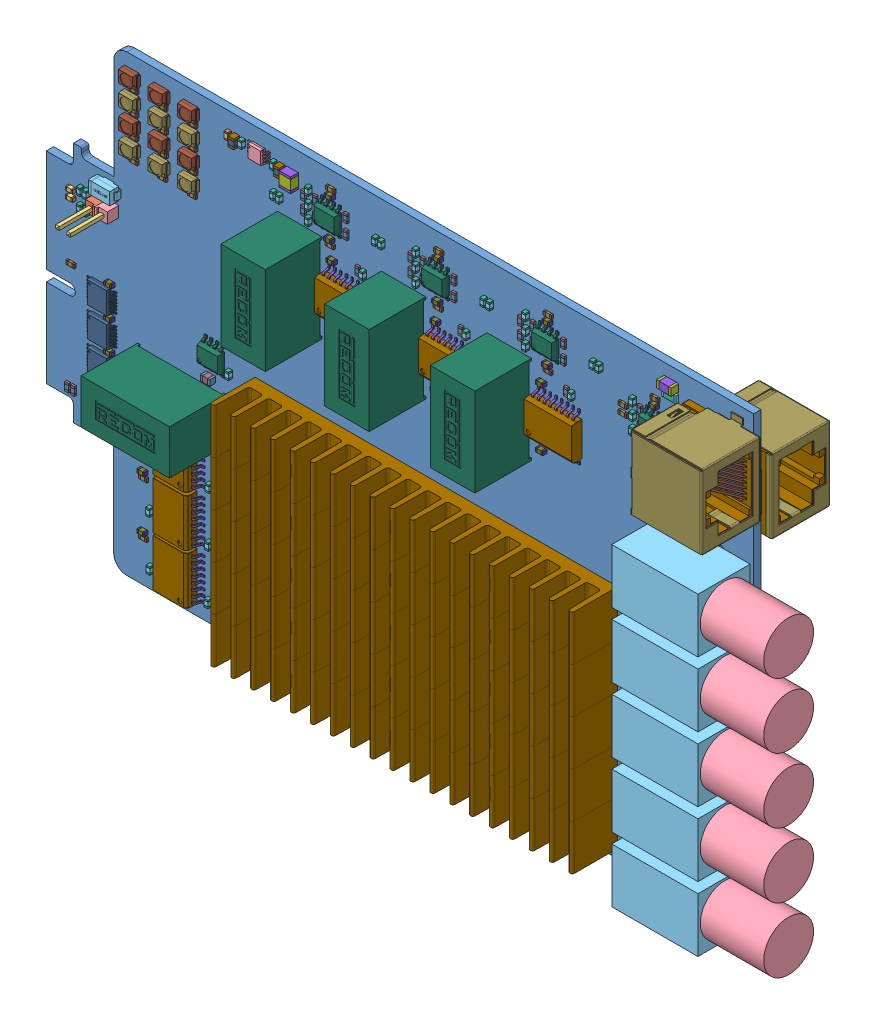
SolidWorks assembly 1166V10, configuration Standard. Lengths in mm.
Overall size (170.01 100 28.53).
2772 component instances, 64 part files, 0 mates.
Components (placement in the parent):
- 1166V10.step-1: 1166V10.step [Standard] at origin size (170.01 100 28.53)
  - Board.step-1: Board.step [Standard] at origin size (155.98 100 1.62)
    - Open CASCADE STEP translator 6.8 1.1.1.step-1: Open CASCADE STEP translator 6.8 1.1.1.step [Standard] at (0 0 -1.622) size (155.98 100 1.62)
  - L103.step-1: L103.step [Standard] at origin size (0.8 1.6 0.8)
    - WE-CBF_0603_CBF.step-1: WE-CBF_0603_CBF.step [Standard] at (40.3999 95.6637 0.4) x (-1 0 0) z (0 0 1) size (0.8 1.6 0.8)
      - L_tende.step-1: L_tende.step [Standard] at (0 -0.5 0) size (0.8 0.3 0.8)
      - L_tende.step-2: L_tende.step [Standard] at (0 0.5 0) x (-1 0 0) z (0 0 1) size (0.8 0.3 0.8)
      - base.step-1: base.step [Standard] at origin size (0.8 1 0.8)
  - IC104.step-1: IC104.step [Standard] at origin size (4.9 3 1.15)
    - MSOP-8.step-1: MSOP-8.step [Standard] at (47.0083 95.5593 0) x (1 0 0) z (0 0 1) size (4.9 3 1.15)
  - CF514.step-1: CF514.step [Standard] at origin size (0.82 1.6 0.9)
    - 6547668352.step-1: 6547668352.step [Standard] at (98.2 92.15 0) size (0.82 0.9 0.9)
      - Extruded.step-1: Extruded.step [Standard] at origin size (0.82 0.9 0.9)
    - 6549602528.step-1: 6549602528.step [Standard] at (98.2 91.525 0) size (0.82 0.35 0.9)
      - Extruded-0.step-1: Extruded-0.step [Standard] at origin size (0.82 0.35 0.9)
    - 6549602528.step-2: 6549602528.step [Standard] at (98.2 92.775 0) size (0.82 0.35 0.9)
      - Extruded-0.step-1: Extruded-0.step [Standard] at origin size (0.82 0.35 0.9)
  - CF513.step-1: CF513.step [Standard] at origin size (0.82 1.6 0.9)
    - 6547668352.step-1: 6547668352.step [Standard] at (96.9 92.15 0) size (0.82 0.9 0.9)
      - Extruded.step-1: Extruded.step [Standard] at origin size (0.82 0.9 0.9)
    - 6549602528.step-1: 6549602528.step [Standard] at (96.9 91.525 0) size (0.82 0.35 0.9)
      - Extruded-0.step-1: Extruded-0.step [Standard] at origin size (0.82 0.35 0.9)
    - 6549602528.step-2: 6549602528.step [Standard] at (96.9 92.775 0) size (0.82 0.35 0.9)
      - Extruded-0.step-1: Extruded-0.step [Standard] at origin size (0.82 0.35 0.9)
  - CF512.step-1: CF512.step [Standard] at origin size (0.82 1.6 0.9)
    - 6547668352.step-1: 6547668352.step [Standard] at (74.3 91.85 0) size (0.82 0.9 0.9)
      - Extruded.step-1: Extruded.step [Standard] at origin size (0.82 0.9 0.9)
    - 6549602528.step-1: 6549602528.step [Standard] at (74.3 91.225 0) size (0.82 0.35 0.9)
      - Extruded-0.step-1: Extruded-0.step [Standard] at origin size (0.82 0.35 0.9)
    - 6549602528.step-2: 6549602528.step [Standard] at (74.3 92.475 0) size (0.82 0.35 0.9)
      - Extruded-0.step-1: Extruded-0.step [Standard] at origin size (0.82 0.35 0.9)
  - CF511.step-1: CF511.step [Standard] at origin size (0.82 1.6 0.9)
    - 6547668352.step-1: 6547668352.step [Standard] at (73 91.85 0) size (0.82 0.9 0.9)
      - Extruded.step-1: Extruded.step [Standard] at origin size (0.82 0.9 0.9)
    - 6549602528.step-1: 6549602528.step [Standard] at (73 91.225 0) size (0.82 0.35 0.9)
      - Extruded-0.step-1: Extruded-0.step [Standard] at origin size (0.82 0.35 0.9)
    - 6549602528.step-2: 6549602528.step [Standard] at (73 92.475 0) size (0.82 0.35 0.9)
      - Extruded-0.step-1: Extruded-0.step [Standard] at origin size (0.82 0.35 0.9)
  - CF510.step-1: CF510.step [Standard] at origin size (0.82 1.6 0.9)
    - 6547668352.step-1: 6547668352.step [Standard] at (122.3 92.25 0) size (0.82 0.9 0.9)
      - Extruded.step-1: Extruded.step [Standard] at origin size (0.82 0.9 0.9)
    - 6549602528.step-1: 6549602528.step [Standard] at (122.3 91.625 0) size (0.82 0.35 0.9)
      - Extruded-0.step-1: Extruded-0.step [Standard] at origin size (0.82 0.35 0.9)
    - 6549602528.step-2: 6549602528.step [Standard] at (122.3 92.875 0) size (0.82 0.35 0.9)
      - Extruded-0.step-1: Extruded-0.step [Standard] at origin size (0.82 0.35 0.9)
  - CF509.step-1: CF509.step [Standard] at origin size (0.82 1.6 0.9)
    - 6547668352.step-1: 6547668352.step [Standard] at (121 92.25 0) size (0.82 0.9 0.9)
      - Extruded.step-1: Extruded.step [Standard] at origin size (0.82 0.9 0.9)
    - 6549602528.step-1: 6549602528.step [Standard] at (121 91.625 0) size (0.82 0.35 0.9)
      - Extruded-0.step-1: Extruded-0.step [Standard] at origin size (0.82 0.35 0.9)
    - 6549602528.step-2: 6549602528.step [Standard] at (121 92.875 0) size (0.82 0.35 0.9)
      - Extruded-0.step-1: Extruded-0.step [Standard] at origin size (0.82 0.35 0.9)
  - CF508.step-1: CF508.step [Standard] at origin size (0.82 1.6 0.9)
    - 6547668352.step-1: 6547668352.step [Standard] at (51.8 89.35 0) size (0.82 0.9 0.9)
      - Extruded.step-1: Extruded.step [Standard] at origin size (0.82 0.9 0.9)
    - 6549602528.step-1: 6549602528.step [Standard] at (51.8 88.725 0) size (0.82 0.35 0.9)
      - Extruded-0.step-1: Extruded-0.step [Standard] at origin size (0.82 0.35 0.9)
    - 6549602528.step-2: 6549602528.step [Standard] at (51.8 89.975 0) size (0.82 0.35 0.9)
      - Extruded-0.step-1: Extruded-0.step [Standard] at origin size (0.82 0.35 0.9)
  - CF507.step-1: CF507.step [Standard] at origin size (0.82 1.6 0.9)
    - 6547668352.step-1: 6547668352.step [Standard] at (50.5 89.35 0) size (0.82 0.9 0.9)
      - Extruded.step-1: Extruded.step [Standard] at origin size (0.82 0.9 0.9)
    - 6549602528.step-1: 6549602528.step [Standard] at (50.5 88.725 0) size (0.82 0.35 0.9)
      - Extruded-0.step-1: Extruded-0.step [Standard] at origin size (0.82 0.35 0.9)
    - 6549602528.step-2: 6549602528.step [Standard] at (50.5 89.975 0) size (0.82 0.35 0.9)
      - Extruded-0.step-1: Extruded-0.step [Standard] at origin size (0.82 0.35 0.9)
  - CF506.step-1: CF506.step [Standard] at origin size (0.82 1.6 0.9)
    - 6549602528.step-1: 6549602528.step [Standard] at (135.1 85.325 -2.522) size (0.82 0.35 0.9)
      - Extruded-0.step-1: Extruded-0.step [Standard] at origin size (0.82 0.35 0.9)
    - 6549602528.step-2: 6549602528.step [Standard] at (135.1 86.575 -2.522) size (0.82 0.35 0.9)
      - Extruded-0.step-1: Extruded-0.step [Standard] at origin size (0.82 0.35 0.9)
    - 6547668352.step-1: 6547668352.step [Standard] at (135.1 85.95 -2.522) size (0.82 0.9 0.9)
      - Extruded.step-1: Extruded.step [Standard] at origin size (0.82 0.9 0.9)
  - CF505.step-1: CF505.step [Standard] at origin size (0.82 1.6 0.9)
    - 6549602528.step-1: 6549602528.step [Standard] at (133.8 85.325 -2.522) size (0.82 0.35 0.9)
      - Extruded-0.step-1: Extruded-0.step [Standard] at origin size (0.82 0.35 0.9)
    - 6549602528.step-2: 6549602528.step [Standard] at (133.8 86.575 -2.522) size (0.82 0.35 0.9)
      - Extruded-0.step-1: Extruded-0.step [Standard] at origin size (0.82 0.35 0.9)
    - 6547668352.step-1: 6547668352.step [Standard] at (133.8 85.95 -2.522) size (0.82 0.9 0.9)
      - Extruded.step-1: Extruded.step [Standard] at origin size (0.82 0.9 0.9)
  - CF412.step-1: CF412.step [Standard] at origin size (0.82 1.6 0.9)
    - 6549602528.step-1: 6549602528.step [Standard] at (63.6 89.525 -2.522) size (0.82 0.35 0.9)
      - Extruded-0.step-1: Extruded-0.step [Standard] at origin size (0.82 0.35 0.9)
    - 6549602528.step-2: 6549602528.step [Standard] at (63.6 90.775 -2.522) size (0.82 0.35 0.9)
      - Extruded-0.step-1: Extruded-0.step [Standard] at origin size (0.82 0.35 0.9)
    - 6547668352.step-1: 6547668352.step [Standard] at (63.6 90.15 -2.522) size (0.82 0.9 0.9)
      - Extruded.step-1: Extruded.step [Standard] at origin size (0.82 0.9 0.9)
  - CF411.step-1: CF411.step [Standard] at origin size (0.82 1.6 0.9)
    - 6549602528.step-1: 6549602528.step [Standard] at (62.3 91.725 -2.522) size (0.82 0.35 0.9)
      - Extruded-0.step-1: Extruded-0.step [Standard] at origin size (0.82 0.35 0.9)
    - 6549602528.step-2: 6549602528.step [Standard] at (62.3 92.975 -2.522) size (0.82 0.35 0.9)
      - Extruded-0.step-1: Extruded-0.step [Standard] at origin size (0.82 0.35 0.9)
    - 6547668352.step-1: 6547668352.step [Standard] at (62.3 92.35 -2.522) size (0.82 0.9 0.9)
      - Extruded.step-1: Extruded.step [Standard] at origin size (0.82 0.9 0.9)
  - CF312.step-1: CF312.step [Standard] at origin size (0.82 1.6 0.9)
    - 6549602528.step-1: 6549602528.step [Standard] at (87.3 89.625 -2.522) size (0.82 0.35 0.9)
      - Extruded-0.step-1: Extruded-0.step [Standard] at origin size (0.82 0.35 0.9)
    - 6549602528.step-2: 6549602528.step [Standard] at (87.3 90.875 -2.522) size (0.82 0.35 0.9)
      - Extruded-0.step-1: Extruded-0.step [Standard] at origin size (0.82 0.35 0.9)
    - 6547668352.step-1: 6547668352.step [Standard] at (87.3 90.25 -2.522) size (0.82 0.9 0.9)
      - Extruded.step-1: Extruded.step [Standard] at origin size (0.82 0.9 0.9)
  - CF311.step-1: CF311.step [Standard] at origin size (0.82 1.6 0.9)
    - 6549602528.step-1: 6549602528.step [Standard] at (86 89.625 -2.522) size (0.82 0.35 0.9)
      - Extruded-0.step-1: Extruded-0.step [Standard] at origin size (0.82 0.35 0.9)
    - 6549602528.step-2: 6549602528.step [Standard] at (86 90.875 -2.522) size (0.82 0.35 0.9)
      - Extruded-0.step-1: Extruded-0.step [Standard] at origin size (0.82 0.35 0.9)
    - 6547668352.step-1: 6547668352.step [Standard] at (86 90.25 -2.522) size (0.82 0.9 0.9)
      - Extruded.step-1: Extruded.step [Standard] at origin size (0.82 0.9 0.9)
  - CF215.step-1: CF215.step [Standard] at origin size (0.82 1.6 0.9)
    - 6549602528.step-1: 6549602528.step [Standard] at (111.5 89.625 -2.522) size (0.82 0.35 0.9)
      - Extruded-0.step-1: Extruded-0.step [Standard] at origin size (0.82 0.35 0.9)
    - 6549602528.step-2: 6549602528.step [Standard] at (111.5 90.875 -2.522) size (0.82 0.35 0.9)
      - Extruded-0.step-1: Extruded-0.step [Standard] at origin size (0.82 0.35 0.9)
    - 6547668352.step-1: 6547668352.step [Standard] at (111.5 90.25 -2.522) size (0.82 0.9 0.9)
      - Extruded.step-1: Extruded.step [Standard] at origin size (0.82 0.9 0.9)
  - CF214.step-1: CF214.step [Standard] at origin size (0.82 1.6 0.9)
    - 6549602528.step-1: 6549602528.step [Standard] at (110.2 89.625 -2.522) size (0.82 0.35 0.9)
      - Extruded-0.step-1: Extruded-0.step [Standard] at origin size (0.82 0.35 0.9)
    - 6549602528.step-2: 6549602528.step [Standard] at (110.2 90.875 -2.522) size (0.82 0.35 0.9)
      - Extruded-0.step-1: Extruded-0.step [Standard] at origin size (0.82 0.35 0.9)
    - 6547668352.step-1: 6547668352.step [Standard] at (110.2 90.25 -2.522) size (0.82 0.9 0.9)
      - Extruded.step-1: Extruded.step [Standard] at origin size (0.82 0.9 0.9)
  - C109.step-1: C109.step [Standard] at origin size (2.5 3.2 1.7)
    - 6547453760.step-1: 6547453760.step [Standard] at (54.3 94.25 0) size (2.5 2.2 1.7)
      - Extruded-1.step-1: Extruded-1.step [Standard] at origin size (2.5 2.2 1.7)
    - 6547453440.step-1: 6547453440.step [Standard] at (54.3 95.6 0) size (2.5 0.5 1.7)
      - Extruded-2.step-1: Extruded-2.step [Standard] at origin size (2.5 0.5 1.7)
    - 6547453440.step-2: 6547453440.step [Standard] at (54.3 92.9 0) size (2.5 0.5 1.7)
      - Extruded-2.step-1: Extruded-2.step [Standard] at origin size (2.5 0.5 1.7)
  - C108.step-1: C108.step [Standard] at origin size (0.82 1.6 0.9)
    - 6549602528.step-1: 6549602528.step [Standard] at (50.5 94.425 0) size (0.82 0.35 0.9)
      - Extruded-0.step-1: Extruded-0.step [Standard] at origin size (0.82 0.35 0.9)
    - 6549602528.step-2: 6549602528.step [Standard] at (50.5 95.675 0) size (0.82 0.35 0.9)
      - Extruded-0.step-1: Extruded-0.step [Standard] at origin size (0.82 0.35 0.9)
    - 6547668352.step-1: 6547668352.step [Standard] at (50.5 95.05 0) size (0.82 0.9 0.9)
      - Extruded.step-1: Extruded.step [Standard] at origin size (0.82 0.9 0.9)
  - C107.step-1: C107.step [Standard] at origin size (1.25 2.1 1.3)
    - 6549603568.step-1: 6549603568.step [Standard] at (52 94 0) size (1.25 0.5 1.3)
      - Extruded-3.step-1: Extruded-3.step [Standard] at origin size (1.25 0.5 1.3)
    - 6549603568.step-2: 6549603568.step [Standard] at (52 95.6 0) size (1.25 0.5 1.3)
      - Extruded-3.step-1: Extruded-3.step [Standard] at origin size (1.25 0.5 1.3)
    - 6549603008.step-1: 6549603008.step [Standard] at (52 94.8 0) size (1.25 1.1 1.3)
      - Extruded-4.step-1: Extruded-4.step [Standard] at origin size (1.25 1.1 1.3)
  - C106.step-1: C106.step [Standard] at origin size (0.82 1.6 0.9)
    - 6549602528.step-1: 6549602528.step [Standard] at (43.5 95.025 0) size (0.82 0.35 0.9)
      - Extruded-0.step-1: Extruded-0.step [Standard] at origin size (0.82 0.35 0.9)
    - 6549602528.step-2: 6549602528.step [Standard] at (43.5 96.275 0) size (0.82 0.35 0.9)
      - Extruded-0.step-1: Extruded-0.step [Standard] at origin size (0.82 0.35 0.9)
    - 6547668352.step-1: 6547668352.step [Standard] at (43.5 95.65 0) size (0.82 0.9 0.9)
      - Extruded.step-1: Extruded.step [Standard] at origin size (0.82 0.9 0.9)
  - C105.step-1: C105.step [Standard] at origin size (1.25 2.1 1.3)
    - 6549603568.step-1: 6549603568.step [Standard] at (42 94.6 0) size (1.25 0.5 1.3)
      - Extruded-3.step-1: Extruded-3.step [Standard] at origin size (1.25 0.5 1.3)
    - 6549603568.step-2: 6549603568.step [Standard] at (42 96.2 0) size (1.25 0.5 1.3)
      - Extruded-3.step-1: Extruded-3.step [Standard] at origin size (1.25 0.5 1.3)
    - 6549603008.step-1: 6549603008.step [Standard] at (42 95.4 0) size (1.25 1.1 1.3)
      - Extruded-4.step-1: Extruded-4.step [Standard] at origin size (1.25 1.1 1.3)
  - R547.step-1: R547.step [Standard] at origin size (1.85 0.85 0.45)
    - 6547171712.step-1: 6547171712.step [Standard] at (96.95 96.6 -2.072) size (0.45 0.85 0.45)
      - Extruded-5.step-1: Extruded-5.step [Standard] at origin size (0.45 0.85 0.45)
    - 6547171712.step-2: 6547171712.step [Standard] at (98.35 96.6 -2.072) size (0.45 0.85 0.45)
      - Extruded-5.step-1: Extruded-5.step [Standard] at origin size (0.45 0.85 0.45)
    - 6547171152.step-1: 6547171152.step [Standard] at (97.65 96.6 -2.072) size (0.95 0.85 0.45)
      - Extruded-6.step-1: Extruded-6.step [Standard] at origin size (0.95 0.85 0.45)
  - R546.step-1: R546.step [Standard] at origin size (0.85 1.85 0.45)
    - 6549605008.step-1: 6549605008.step [Standard] at (91.4 91.65 -2.072) size (0.85 0.45 0.45)
      - Extruded-7.step-1: Extruded-7.step [Standard] at origin size (0.85 0.45 0.45)
    - 6549605008.step-2: 6549605008.step [Standard] at (91.4 93.05 -2.072) size (0.85 0.45 0.45)
      - Extruded-7.step-1: Extruded-7.step [Standard] at origin size (0.85 0.45 0.45)
    - 6549605488.step-1: 6549605488.step [Standard] at (91.4 92.35 -2.072) size (0.85 0.95 0.45)
      - Extruded-8.step-1: Extruded-8.step [Standard] at origin size (0.85 0.95 0.45)
  - R545.step-1: R545.step [Standard] at origin size (0.85 1.85 0.45)
    - 6549605008.step-1: 6549605008.step [Standard] at (94.1 92.15 -2.072) size (0.85 0.45 0.45)
      - Extruded-7.step-1: Extruded-7.step [Standard] at origin size (0.85 0.45 0.45)
    - 6549605008.step-2: 6549605008.step [Standard] at (94.1 93.55 -2.072) size (0.85 0.45 0.45)
      - Extruded-7.step-1: Extruded-7.step [Standard] at origin size (0.85 0.45 0.45)
    - 6549605488.step-1: 6549605488.step [Standard] at (94.1 92.85 -2.072) size (0.85 0.95 0.45)
      - Extruded-8.step-1: Extruded-8.step [Standard] at origin size (0.85 0.95 0.45)
  - R544.step-1: R544.step [Standard] at origin size (0.85 1.85 0.45)
    - 6549605008.step-1: 6549605008.step [Standard] at (100.9 93.55 -2.072) size (0.85 0.45 0.45)
      - Extruded-7.step-1: Extruded-7.step [Standard] at origin size (0.85 0.45 0.45)
    - 6549605008.step-2: 6549605008.step [Standard] at (100.9 92.15 -2.072) size (0.85 0.45 0.45)
      - Extruded-7.step-1: Extruded-7.step [Standard] at origin size (0.85 0.45 0.45)
    - 6549605488.step-1: 6549605488.step [Standard] at (100.9 92.85 -2.072) size (0.85 0.95 0.45)
      - Extruded-8.step-1: Extruded-8.step [Standard] at origin size (0.85 0.95 0.45)
  - R543.step-1: R543.step [Standard] at origin size (0.85 1.85 0.45)
    - 6549605008.step-1: 6549605008.step [Standard] at (91.4 88.75 -2.072) size (0.85 0.45 0.45)
      - Extruded-7.step-1: Extruded-7.step [Standard] at origin size (0.85 0.45 0.45)
    - 6549605008.step-2: 6549605008.step [Standard] at (91.4 90.15 -2.072) size (0.85 0.45 0.45)
      - Extruded-7.step-1: Extruded-7.step [Standard] at origin size (0.85 0.45 0.45)
    - 6549605488.step-1: 6549605488.step [Standard] at (91.4 89.45 -2.072) size (0.85 0.95 0.45)
      - Extruded-8.step-1: Extruded-8.step [Standard] at origin size (0.85 0.95 0.45)
  - R542.step-1: R542.step [Standard] at origin size (0.85 1.85 0.45)
    - 6549605008.step-1: 6549605008.step [Standard] at (94.1 90.35 -2.072) size (0.85 0.45 0.45)
      - Extruded-7.step-1: Extruded-7.step [Standard] at origin size (0.85 0.45 0.45)
    - 6549605008.step-2: 6549605008.step [Standard] at (94.1 88.95 -2.072) size (0.85 0.45 0.45)
      - Extruded-7.step-1: Extruded-7.step [Standard] at origin size (0.85 0.45 0.45)
    - 6549605488.step-1: 6549605488.step [Standard] at (94.1 89.65 -2.072) size (0.85 0.95 0.45)
      - Extruded-8.step-1: Extruded-8.step [Standard] at origin size (0.85 0.95 0.45)
  - R541.step-1: R541.step [Standard] at origin size (0.85 1.85 0.45)
    - 6549605008.step-1: 6549605008.step [Standard] at (100.9 88.95 -2.072) size (0.85 0.45 0.45)
      - Extruded-7.step-1: Extruded-7.step [Standard] at origin size (0.85 0.45 0.45)
    - 6549605008.step-2: 6549605008.step [Standard] at (100.9 90.35 -2.072) size (0.85 0.45 0.45)
      - Extruded-7.step-1: Extruded-7.step [Standard] at origin size (0.85 0.45 0.45)
    - 6549605488.step-1: 6549605488.step [Standard] at (100.9 89.65 -2.072) size (0.85 0.95 0.45)
      - Extruded-8.step-1: Extruded-8.step [Standard] at origin size (0.85 0.95 0.45)
  - R540.step-1: R540.step [Standard] at origin size (1.85 0.85 0.45)
    - 6547171712.step-1: 6547171712.step [Standard] at (73.05 96.3 -2.072) size (0.45 0.85 0.45)
      - Extruded-5.step-1: Extruded-5.step [Standard] at origin size (0.45 0.85 0.45)
    - 6547171712.step-2: 6547171712.step [Standard] at (74.45 96.3 -2.072) size (0.45 0.85 0.45)
      - Extruded-5.step-1: Extruded-5.step [Standard] at origin size (0.45 0.85 0.45)
    - 6547171152.step-1: 6547171152.step [Standard] at (73.75 96.3 -2.072) size (0.95 0.85 0.45)
      - Extruded-6.step-1: Extruded-6.step [Standard] at origin size (0.95 0.85 0.45)
  - R539.step-1: R539.step [Standard] at origin size (1.85 0.85 0.45)
    - 6547171712.step-1: 6547171712.step [Standard] at (96.85 85.9 -2.072) size (0.45 0.85 0.45)
      - Extruded-5.step-1: Extruded-5.step [Standard] at origin size (0.45 0.85 0.45)
    - 6547171712.step-2: 6547171712.step [Standard] at (98.25 85.9 -2.072) size (0.45 0.85 0.45)
      - Extruded-5.step-1: Extruded-5.step [Standard] at origin size (0.45 0.85 0.45)
    - 6547171152.step-1: 6547171152.step [Standard] at (97.55 85.9 -2.072) size (0.95 0.85 0.45)
      - Extruded-6.step-1: Extruded-6.step [Standard] at origin size (0.95 0.85 0.45)
  - R538.step-1: R538.step [Standard] at origin size (0.85 1.85 0.45)
    - 6549605008.step-1: 6549605008.step [Standard] at (67.6 91.35 -2.072) size (0.85 0.45 0.45)
      - Extruded-7.step-1: Extruded-7.step [Standard] at origin size (0.85 0.45 0.45)
    - 6549605008.step-2: 6549605008.step [Standard] at (67.6 92.75 -2.072) size (0.85 0.45 0.45)
      - Extruded-7.step-1: Extruded-7.step [Standard] at origin size (0.85 0.45 0.45)
    - 6549605488.step-1: 6549605488.step [Standard] at (67.6 92.05 -2.072) size (0.85 0.95 0.45)
      - Extruded-8.step-1: Extruded-8.step [Standard] at origin size (0.85 0.95 0.45)
  - R537.step-1: R537.step [Standard] at origin size (0.85 1.85 0.45)
    - 6549605008.step-1: 6549605008.step [Standard] at (70.3 91.85 -2.072) size (0.85 0.45 0.45)
      - Extruded-7.step-1: Extruded-7.step [Standard] at origin size (0.85 0.45 0.45)
    - 6549605008.step-2: 6549605008.step [Standard] at (70.3 93.25 -2.072) size (0.85 0.45 0.45)
      - Extruded-7.step-1: Extruded-7.step [Standard] at origin size (0.85 0.45 0.45)
    - 6549605488.step-1: 6549605488.step [Standard] at (70.3 92.55 -2.072) size (0.85 0.95 0.45)
      - Extruded-8.step-1: Extruded-8.step [Standard] at origin size (0.85 0.95 0.45)
  - R536.step-1: R536.step [Standard] at origin size (0.85 1.85 0.45)
    - 6549605008.step-1: 6549605008.step [Standard] at (77.1 93.25 -2.072) size (0.85 0.45 0.45)
      - Extruded-7.step-1: Extruded-7.step [Standard] at origin size (0.85 0.45 0.45)
    - 6549605008.step-2: 6549605008.step [Standard] at (77.1 91.85 -2.072) size (0.85 0.45 0.45)
      - Extruded-7.step-1: Extruded-7.step [Standard] at origin size (0.85 0.45 0.45)
    - 6549605488.step-1: 6549605488.step [Standard] at (77.1 92.55 -2.072) size (0.85 0.95 0.45)
      - Extruded-8.step-1: Extruded-8.step [Standard] at origin size (0.85 0.95 0.45)
  - R535.step-1: R535.step [Standard] at origin size (1.85 0.85 0.45)
    - 6547171712.step-1: 6547171712.step [Standard] at (121.05 96.7 -2.072) size (0.45 0.85 0.45)
      - Extruded-5.step-1: Extruded-5.step [Standard] at origin size (0.45 0.85 0.45)
    - 6547171712.step-2: 6547171712.step [Standard] at (122.45 96.7 -2.072) size (0.45 0.85 0.45)
      - Extruded-5.step-1: Extruded-5.step [Standard] at origin size (0.45 0.85 0.45)
    - 6547171152.step-1: 6547171152.step [Standard] at (121.75 96.7 -2.072) size (0.95 0.85 0.45)
      - Extruded-6.step-1: Extruded-6.step [Standard] at origin size (0.95 0.85 0.45)
  - R534.step-1: R534.step [Standard] at origin size (0.85 1.85 0.45)
    - 6549605008.step-1: 6549605008.step [Standard] at (67.6 88.45 -2.072) size (0.85 0.45 0.45)
      - Extruded-7.step-1: Extruded-7.step [Standard] at origin size (0.85 0.45 0.45)
    - 6549605008.step-2: 6549605008.step [Standard] at (67.6 89.85 -2.072) size (0.85 0.45 0.45)
      - Extruded-7.step-1: Extruded-7.step [Standard] at origin size (0.85 0.45 0.45)
    - 6549605488.step-1: 6549605488.step [Standard] at (67.6 89.15 -2.072) size (0.85 0.95 0.45)
      - Extruded-8.step-1: Extruded-8.step [Standard] at origin size (0.85 0.95 0.45)
  - R533.step-1: R533.step [Standard] at origin size (0.85 1.85 0.45)
    - 6549605008.step-1: 6549605008.step [Standard] at (70.3 90.05 -2.072) size (0.85 0.45 0.45)
      - Extruded-7.step-1: Extruded-7.step [Standard] at origin size (0.85 0.45 0.45)
    - 6549605008.step-2: 6549605008.step [Standard] at (70.3 88.65 -2.072) size (0.85 0.45 0.45)
      - Extruded-7.step-1: Extruded-7.step [Standard] at origin size (0.85 0.45 0.45)
    - 6549605488.step-1: 6549605488.step [Standard] at (70.3 89.35 -2.072) size (0.85 0.95 0.45)
      - Extruded-8.step-1: Extruded-8.step [Standard] at origin size (0.85 0.95 0.45)
  - R532.step-1: R532.step [Standard] at origin size (0.85 1.85 0.45)
    - 6549605008.step-1: 6549605008.step [Standard] at (77.1 88.65 -2.072) size (0.85 0.45 0.45)
      - Extruded-7.step-1: Extruded-7.step [Standard] at origin size (0.85 0.45 0.45)
    - 6549605008.step-2: 6549605008.step [Standard] at (77.1 90.05 -2.072) size (0.85 0.45 0.45)
      - Extruded-7.step-1: Extruded-7.step [Standard] at origin size (0.85 0.45 0.45)
    - 6549605488.step-1: 6549605488.step [Standard] at (77.1 89.35 -2.072) size (0.85 0.95 0.45)
      - Extruded-8.step-1: Extruded-8.step [Standard] at origin size (0.85 0.95 0.45)
  - R531.step-1: R531.step [Standard] at origin size (0.85 1.85 0.45)
    - 6549605008.step-1: 6549605008.step [Standard] at (115.6 92.05 -2.072) size (0.85 0.45 0.45)
      - Extruded-7.step-1: Extruded-7.step [Standard] at origin size (0.85 0.45 0.45)
    - 6549605008.step-2: 6549605008.step [Standard] at (115.6 93.45 -2.072) size (0.85 0.45 0.45)
      - Extruded-7.step-1: Extruded-7.step [Standard] at origin size (0.85 0.45 0.45)
    - 6549605488.step-1: 6549605488.step [Standard] at (115.6 92.75 -2.072) size (0.85 0.95 0.45)
      - Extruded-8.step-1: Extruded-8.step [Standard] at origin size (0.85 0.95 0.45)
  - R530.step-1: R530.step [Standard] at origin size (0.85 1.85 0.45)
    - 6549605008.step-1: 6549605008.step [Standard] at (118.3 92.25 -2.072) size (0.85 0.45 0.45)
      - Extruded-7.step-1: Extruded-7.step [Standard] at origin size (0.85 0.45 0.45)
    - 6549605008.step-2: 6549605008.step [Standard] at (118.3 93.65 -2.072) size (0.85 0.45 0.45)
      - Extruded-7.step-1: Extruded-7.step [Standard] at origin size (0.85 0.45 0.45)
    - 6549605488.step-1: 6549605488.step [Standard] at (118.3 92.95 -2.072) size (0.85 0.95 0.45)
      - Extruded-8.step-1: Extruded-8.step [Standard] at origin size (0.85 0.95 0.45)
  - R529.step-1: R529.step [Standard] at origin size (0.85 1.85 0.45)
    - 6549605008.step-1: 6549605008.step [Standard] at (125.07 93.65 -2.072) size (0.85 0.45 0.45)
      - Extruded-7.step-1: Extruded-7.step [Standard] at origin size (0.85 0.45 0.45)
    - 6549605008.step-2: 6549605008.step [Standard] at (125.07 92.25 -2.072) size (0.85 0.45 0.45)
      - Extruded-7.step-1: Extruded-7.step [Standard] at origin size (0.85 0.45 0.45)
    - 6549605488.step-1: 6549605488.step [Standard] at (125.07 92.95 -2.072) size (0.85 0.95 0.45)
      - Extruded-8.step-1: Extruded-8.step [Standard] at origin size (0.85 0.95 0.45)
  - R528.step-1: R528.step [Standard] at origin size (1.85 0.85 0.45)
    - 6547171712.step-1: 6547171712.step [Standard] at (73.05 85.6 -2.072) size (0.45 0.85 0.45)
      - Extruded-5.step-1: Extruded-5.step [Standard] at origin size (0.45 0.85 0.45)
    - 6547171712.step-2: 6547171712.step [Standard] at (74.45 85.6 -2.072) size (0.45 0.85 0.45)
      - Extruded-5.step-1: Extruded-5.step [Standard] at origin size (0.45 0.85 0.45)
    - 6547171152.step-1: 6547171152.step [Standard] at (73.75 85.6 -2.072) size (0.95 0.85 0.45)
      - Extruded-6.step-1: Extruded-6.step [Standard] at origin size (0.95 0.85 0.45)
  - R527.step-1: R527.step [Standard] at origin size (0.85 1.85 0.45)
    - 6549605008.step-1: 6549605008.step [Standard] at (115.6 89.15 -2.072) size (0.85 0.45 0.45)
      - Extruded-7.step-1: Extruded-7.step [Standard] at origin size (0.85 0.45 0.45)
    - 6549605008.step-2: 6549605008.step [Standard] at (115.6 90.55 -2.072) size (0.85 0.45 0.45)
      - Extruded-7.step-1: Extruded-7.step [Standard] at origin size (0.85 0.45 0.45)
    - 6549605488.step-1: 6549605488.step [Standard] at (115.6 89.85 -2.072) size (0.85 0.95 0.45)
      - Extruded-8.step-1: Extruded-8.step [Standard] at origin size (0.85 0.95 0.45)
  - R526.step-1: R526.step [Standard] at origin size (0.85 1.85 0.45)
    - 6549605008.step-1: 6549605008.step [Standard] at (118.3 90.45 -2.072) size (0.85 0.45 0.45)
      - Extruded-7.step-1: Extruded-7.step [Standard] at origin size (0.85 0.45 0.45)
    - 6549605008.step-2: 6549605008.step [Standard] at (118.3 89.05 -2.072) size (0.85 0.45 0.45)
      - Extruded-7.step-1: Extruded-7.step [Standard] at origin size (0.85 0.45 0.45)
    - 6549605488.step-1: 6549605488.step [Standard] at (118.3 89.75 -2.072) size (0.85 0.95 0.45)
      - Extruded-8.step-1: Extruded-8.step [Standard] at origin size (0.85 0.95 0.45)
  - R525.step-1: R525.step [Standard] at origin size (0.85 1.85 0.45)
    - 6549605008.step-1: 6549605008.step [Standard] at (125.07 89.05 -2.072) size (0.85 0.45 0.45)
      - Extruded-7.step-1: Extruded-7.step [Standard] at origin size (0.85 0.45 0.45)
    - 6549605008.step-2: 6549605008.step [Standard] at (125.07 90.45 -2.072) size (0.85 0.45 0.45)
      - Extruded-7.step-1: Extruded-7.step [Standard] at origin size (0.85 0.45 0.45)
    - 6549605488.step-1: 6549605488.step [Standard] at (125.07 89.75 -2.072) size (0.85 0.95 0.45)
      - Extruded-8.step-1: Extruded-8.step [Standard] at origin size (0.85 0.95 0.45)
  - R524.step-1: R524.step [Standard] at origin size (1.85 0.85 0.45)
    - 6547171712.step-1: 6547171712.step [Standard] at (120.95 86 -2.072) size (0.45 0.85 0.45)
      - Extruded-5.step-1: Extruded-5.step [Standard] at origin size (0.45 0.85 0.45)
    - 6547171712.step-2: 6547171712.step [Standard] at (122.35 86 -2.072) size (0.45 0.85 0.45)
      - Extruded-5.step-1: Extruded-5.step [Standard] at origin size (0.45 0.85 0.45)
    - 6547171152.step-1: 6547171152.step [Standard] at (121.65 86 -2.072) size (0.95 0.85 0.45)
      - Extruded-6.step-1: Extruded-6.step [Standard] at origin size (0.95 0.85 0.45)
  - R523.step-1: R523.step [Standard] at origin size (1.85 0.85 0.45)
    - 6547171712.step-1: 6547171712.step [Standard] at (50.45 93.8 -2.072) size (0.45 0.85 0.45)
      - Extruded-5.step-1: Extruded-5.step [Standard] at origin size (0.45 0.85 0.45)
    - 6547171712.step-2: 6547171712.step [Standard] at (51.85 93.8 -2.072) size (0.45 0.85 0.45)
      - Extruded-5.step-1: Extruded-5.step [Standard] at origin size (0.45 0.85 0.45)
    - 6547171152.step-1: 6547171152.step [Standard] at (51.15 93.8 -2.072) size (0.95 0.85 0.45)
      - Extruded-6.step-1: Extruded-6.step [Standard] at origin size (0.95 0.85 0.45)
  - R522.step-1: R522.step [Standard] at origin size (0.85 1.85 0.45)
    - 6549605008.step-1: 6549605008.step [Standard] at (44.9 88.95 -2.072) size (0.85 0.45 0.45)
      - Extruded-7.step-1: Extruded-7.step [Standard] at origin size (0.85 0.45 0.45)
    - 6549605008.step-2: 6549605008.step [Standard] at (44.9 90.35 -2.072) size (0.85 0.45 0.45)
      - Extruded-7.step-1: Extruded-7.step [Standard] at origin size (0.85 0.45 0.45)
    - 6549605488.step-1: 6549605488.step [Standard] at (44.9 89.65 -2.072) size (0.85 0.95 0.45)
      - Extruded-8.step-1: Extruded-8.step [Standard] at origin size (0.85 0.95 0.45)
  - R521.step-1: R521.step [Standard] at origin size (0.85 1.85 0.45)
    - 6549605008.step-1: 6549605008.step [Standard] at (47.7 89.35 -2.072) size (0.85 0.45 0.45)
      - Extruded-7.step-1: Extruded-7.step [Standard] at origin size (0.85 0.45 0.45)
    - 6549605008.step-2: 6549605008.step [Standard] at (47.7 90.75 -2.072) size (0.85 0.45 0.45)
      - Extruded-7.step-1: Extruded-7.step [Standard] at origin size (0.85 0.45 0.45)
    - 6549605488.step-1: 6549605488.step [Standard] at (47.7 90.05 -2.072) size (0.85 0.95 0.45)
      - Extruded-8.step-1: Extruded-8.step [Standard] at origin size (0.85 0.95 0.45)
  - R520.step-1: R520.step [Standard] at origin size (0.85 1.85 0.45)
    - 6549605008.step-1: 6549605008.step [Standard] at (54.6 90.75 -2.072) size (0.85 0.45 0.45)
      - Extruded-7.step-1: Extruded-7.step [Standard] at origin size (0.85 0.45 0.45)
    - 6549605008.step-2: 6549605008.step [Standard] at (54.6 89.35 -2.072) size (0.85 0.45 0.45)
      - Extruded-7.step-1: Extruded-7.step [Standard] at origin size (0.85 0.45 0.45)
    - 6549605488.step-1: 6549605488.step [Standard] at (54.6 90.05 -2.072) size (0.85 0.95 0.45)
      - Extruded-8.step-1: Extruded-8.step [Standard] at origin size (0.85 0.95 0.45)
  - R519.step-1: R519.step [Standard] at origin size (0.85 1.85 0.45)
    - 6549605008.step-1: 6549605008.step [Standard] at (44.9 86.05 -2.072) size (0.85 0.45 0.45)
      - Extruded-7.step-1: Extruded-7.step [Standard] at origin size (0.85 0.45 0.45)
    - 6549605008.step-2: 6549605008.step [Standard] at (44.9 87.45 -2.072) size (0.85 0.45 0.45)
      - Extruded-7.step-1: Extruded-7.step [Standard] at origin size (0.85 0.45 0.45)
    - 6549605488.step-1: 6549605488.step [Standard] at (44.9 86.75 -2.072) size (0.85 0.95 0.45)
      - Extruded-8.step-1: Extruded-8.step [Standard] at origin size (0.85 0.95 0.45)
  - R518.step-1: R518.step [Standard] at origin size (0.85 1.85 0.45)
    - 6549605008.step-1: 6549605008.step [Standard] at (47.7 87.55 -2.072) size (0.85 0.45 0.45)
      - Extruded-7.step-1: Extruded-7.step [Standard] at origin size (0.85 0.45 0.45)
    - 6549605008.step-2: 6549605008.step [Standard] at (47.7 86.15 -2.072) size (0.85 0.45 0.45)
      - Extruded-7.step-1: Extruded-7.step [Standard] at origin size (0.85 0.45 0.45)
    - 6549605488.step-1: 6549605488.step [Standard] at (47.7 86.85 -2.072) size (0.85 0.95 0.45)
      - Extruded-8.step-1: Extruded-8.step [Standard] at origin size (0.85 0.95 0.45)
  - R517.step-1: R517.step [Standard] at origin size (0.85 1.85 0.45)
    - 6549605008.step-1: 6549605008.step [Standard] at (54.6 86.05 -2.072) size (0.85 0.45 0.45)
      - Extruded-7.step-1: Extruded-7.step [Standard] at origin size (0.85 0.45 0.45)
    - 6549605008.step-2: 6549605008.step [Standard] at (54.6 87.45 -2.072) size (0.85 0.45 0.45)
      - Extruded-7.step-1: Extruded-7.step [Standard] at origin size (0.85 0.45 0.45)
    - 6549605488.step-1: 6549605488.step [Standard] at (54.6 86.75 -2.072) size (0.85 0.95 0.45)
      - Extruded-8.step-1: Extruded-8.step [Standard] at origin size (0.85 0.95 0.45)
  - R516.step-1: R516.step [Standard] at origin size (1.85 0.85 0.45)
    - 6547171712.step-1: 6547171712.step [Standard] at (50.45 83.1 -2.072) size (0.45 0.85 0.45)
      - Extruded-5.step-1: Extruded-5.step [Standard] at origin size (0.45 0.85 0.45)
    - 6547171712.step-2: 6547171712.step [Standard] at (51.85 83.1 -2.072) size (0.45 0.85 0.45)
      - Extruded-5.step-1: Extruded-5.step [Standard] at origin size (0.45 0.85 0.45)
    - 6547171152.step-1: 6547171152.step [Standard] at (51.15 83.1 -2.072) size (0.95 0.85 0.45)
      - Extruded-6.step-1: Extruded-6.step [Standard] at origin size (0.95 0.85 0.45)
  - R515.step-1: R515.step [Standard] at origin size (1.85 0.85 0.45)
    - 6547171712.step-1: 6547171712.step [Standard] at (133.75 81.4 0) size (0.45 0.85 0.45)
      - Extruded-5.step-1: Extruded-5.step [Standard] at origin size (0.45 0.85 0.45)
    - 6547171712.step-2: 6547171712.step [Standard] at (135.15 81.4 0) size (0.45 0.85 0.45)
      - Extruded-5.step-1: Extruded-5.step [Standard] at origin size (0.45 0.85 0.45)
    - 6547171152.step-1: 6547171152.step [Standard] at (134.45 81.4 0) size (0.95 0.85 0.45)
      - Extruded-6.step-1: Extruded-6.step [Standard] at origin size (0.95 0.85 0.45)
  - R514.step-1: R514.step [Standard] at origin size (1.85 0.85 0.45)
    - 6547171712.step-1: 6547171712.step [Standard] at (126.75 85.9 0) size (0.45 0.85 0.45)
      - Extruded-5.step-1: Extruded-5.step [Standard] at origin size (0.45 0.85 0.45)
    - 6547171712.step-2: 6547171712.step [Standard] at (128.15 85.9 0) size (0.45 0.85 0.45)
      - Extruded-5.step-1: Extruded-5.step [Standard] at origin size (0.45 0.85 0.45)
    - 6547171152.step-1: 6547171152.step [Standard] at (127.45 85.9 0) size (0.95 0.85 0.45)
      - Extruded-6.step-1: Extruded-6.step [Standard] at origin size (0.95 0.85 0.45)
  - R513.step-1: R513.step [Standard] at origin size (0.85 1.85 0.45)
    - 6549605008.step-1: 6549605008.step [Standard] at (131.1 85.95 0) size (0.85 0.45 0.45)
      - Extruded-7.step-1: Extruded-7.step [Standard] at origin size (0.85 0.45 0.45)
    - 6549605008.step-2: 6549605008.step [Standard] at (131.1 84.55 0) size (0.85 0.45 0.45)
      - Extruded-7.step-1: Extruded-7.step [Standard] at origin size (0.85 0.45 0.45)
    - 6549605488.step-1: 6549605488.step [Standard] at (131.1 85.25 0) size (0.85 0.95 0.45)
      - Extruded-8.step-1: Extruded-8.step [Standard] at origin size (0.85 0.95 0.45)
  - R512.step-1: R512.step [Standard] at origin size (0.85 1.85 0.45)
    - 6549605008.step-1: 6549605008.step [Standard] at (137.9 84.55 0) size (0.85 0.45 0.45)
      - Extruded-7.step-1: Extruded-7.step [Standard] at origin size (0.85 0.45 0.45)
    - 6549605008.step-2: 6549605008.step [Standard] at (137.9 85.95 0) size (0.85 0.45 0.45)
      - Extruded-7.step-1: Extruded-7.step [Standard] at origin size (0.85 0.45 0.45)
    - 6549605488.step-1: 6549605488.step [Standard] at (137.9 85.25 0) size (0.85 0.95 0.45)
      - Extruded-8.step-1: Extruded-8.step [Standard] at origin size (0.85 0.95 0.45)
  - R511.step-1: R511.step [Standard] at origin size (1.85 0.85 0.45)
    - 6547171712.step-1: 6547171712.step [Standard] at (126.75 87.6 0) size (0.45 0.85 0.45)
      - Extruded-5.step-1: Extruded-5.step [Standard] at origin size (0.45 0.85 0.45)
    - 6547171712.step-2: 6547171712.step [Standard] at (128.15 87.6 0) size (0.45 0.85 0.45)
      - Extruded-5.step-1: Extruded-5.step [Standard] at origin size (0.45 0.85 0.45)
    - 6547171152.step-1: 6547171152.step [Standard] at (127.45 87.6 0) size (0.95 0.85 0.45)
      - Extruded-6.step-1: Extruded-6.step [Standard] at origin size (0.95 0.85 0.45)
  - R510.step-1: R510.step [Standard] at origin size (0.85 1.85 0.45)
    - 6549605008.step-1: 6549605008.step [Standard] at (131.1 87.75 0) size (0.85 0.45 0.45)
      - Extruded-7.step-1: Extruded-7.step [Standard] at origin size (0.85 0.45 0.45)
    - 6549605008.step-2: 6549605008.step [Standard] at (131.1 89.15 0) size (0.85 0.45 0.45)
      - Extruded-7.step-1: Extruded-7.step [Standard] at origin size (0.85 0.45 0.45)
    - 6549605488.step-1: 6549605488.step [Standard] at (131.1 88.45 0) size (0.85 0.95 0.45)
      - Extruded-8.step-1: Extruded-8.step [Standard] at origin size (0.85 0.95 0.45)
  - R509.step-1: R509.step [Standard] at origin size (0.85 1.85 0.45)
    - 6549605008.step-1: 6549605008.step [Standard] at (137.9 89.15 0) size (0.85 0.45 0.45)
      - Extruded-7.step-1: Extruded-7.step [Standard] at origin size (0.85 0.45 0.45)
    - 6549605008.step-2: 6549605008.step [Standard] at (137.9 87.75 0) size (0.85 0.45 0.45)
      - Extruded-7.step-1: Extruded-7.step [Standard] at origin size (0.85 0.45 0.45)
    - 6549605488.step-1: 6549605488.step [Standard] at (137.9 88.45 0) size (0.85 0.95 0.45)
      - Extruded-8.step-1: Extruded-8.step [Standard] at origin size (0.85 0.95 0.45)
  - R507.step-1: R507.step [Standard] at origin size (1.85 0.85 0.45)
    - 6547171712.step-1: 6547171712.step [Standard] at (133.75 92.3 0) size (0.45 0.85 0.45)
      - Extruded-5.step-1: Extruded-5.step [Standard] at origin size (0.45 0.85 0.45)
    - 6547171712.step-2: 6547171712.step [Standard] at (135.15 92.3 0) size (0.45 0.85 0.45)
      - Extruded-5.step-1: Extruded-5.step [Standard] at origin size (0.45 0.85 0.45)
    - 6547171152.step-1: 6547171152.step [Standard] at (134.45 92.3 0) size (0.95 0.85 0.45)
      - Extruded-6.step-1: Extruded-6.step [Standard] at origin size (0.95 0.85 0.45)
  - R425.step-1: R425.step [Standard] at origin size (1.85 0.85 0.45)
    - 6547171712.step-1: 6547171712.step [Standard] at (62.16 85.8 0) size (0.45 0.85 0.45)
      - Extruded-5.step-1: Extruded-5.step [Standard] at origin size (0.45 0.85 0.45)
    - 6547171712.step-2: 6547171712.step [Standard] at (63.56 85.8 0) size (0.45 0.85 0.45)
      - Extruded-5.step-1: Extruded-5.step [Standard] at origin size (0.45 0.85 0.45)
    - 6547171152.step-1: 6547171152.step [Standard] at (62.86 85.8 0) size (0.95 0.85 0.45)
      - Extruded-6.step-1: Extruded-6.step [Standard] at origin size (0.95 0.85 0.45)
  - R424.step-1: R424.step [Standard] at origin size (0.85 1.85 0.45)
    - 6549605008.step-1: 6549605008.step [Standard] at (56.91 88.75 0) size (0.85 0.45 0.45)
      - Extruded-7.step-1: Extruded-7.step [Standard] at origin size (0.85 0.45 0.45)
    - 6549605008.step-2: 6549605008.step [Standard] at (56.91 90.15 0) size (0.85 0.45 0.45)
      - Extruded-7.step-1: Extruded-7.step [Standard] at origin size (0.85 0.45 0.45)
    - 6549605488.step-1: 6549605488.step [Standard] at (56.91 89.45 0) size (0.85 0.95 0.45)
      - Extruded-8.step-1: Extruded-8.step [Standard] at origin size (0.85 0.95 0.45)
  - R423.step-1: R423.step [Standard] at origin size (0.85 1.85 0.45)
    - 6549605008.step-1: 6549605008.step [Standard] at (59.51 90.25 0) size (0.85 0.45 0.45)
      - Extruded-7.step-1: Extruded-7.step [Standard] at origin size (0.85 0.45 0.45)
    - 6549605008.step-2: 6549605008.step [Standard] at (59.51 88.85 0) size (0.85 0.45 0.45)
      - Extruded-7.step-1: Extruded-7.step [Standard] at origin size (0.85 0.45 0.45)
    - 6549605488.step-1: 6549605488.step [Standard] at (59.51 89.55 0) size (0.85 0.95 0.45)
      - Extruded-8.step-1: Extruded-8.step [Standard] at origin size (0.85 0.95 0.45)
  - R422.step-1: R422.step [Standard] at origin size (0.85 1.85 0.45)
    - 6549605008.step-1: 6549605008.step [Standard] at (66.31 88.85 0) size (0.85 0.45 0.45)
      - Extruded-7.step-1: Extruded-7.step [Standard] at origin size (0.85 0.45 0.45)
    - 6549605008.step-2: 6549605008.step [Standard] at (66.31 90.25 0) size (0.85 0.45 0.45)
      - Extruded-7.step-1: Extruded-7.step [Standard] at origin size (0.85 0.45 0.45)
    - 6549605488.step-1: 6549605488.step [Standard] at (66.31 89.55 0) size (0.85 0.95 0.45)
      - Extruded-8.step-1: Extruded-8.step [Standard] at origin size (0.85 0.95 0.45)
  - R421.step-1: R421.step [Standard] at origin size (0.85 1.85 0.45)
    - 6549605008.step-1: 6549605008.step [Standard] at (56.91 91.65 0) size (0.85 0.45 0.45)
      - Extruded-7.step-1: Extruded-7.step [Standard] at origin size (0.85 0.45 0.45)
    - 6549605008.step-2: 6549605008.step [Standard] at (56.91 93.05 0) size (0.85 0.45 0.45)
      - Extruded-7.step-1: Extruded-7.step [Standard] at origin size (0.85 0.45 0.45)
    - 6549605488.step-1: 6549605488.step [Standard] at (56.91 92.35 0) size (0.85 0.95 0.45)
      - Extruded-8.step-1: Extruded-8.step [Standard] at origin size (0.85 0.95 0.45)
  - R420.step-1: R420.step [Standard] at origin size (0.85 1.85 0.45)
    - 6549605008.step-1: 6549605008.step [Standard] at (59.51 92.05 0) size (0.85 0.45 0.45)
      - Extruded-7.step-1: Extruded-7.step [Standard] at origin size (0.85 0.45 0.45)
    - 6549605008.step-2: 6549605008.step [Standard] at (59.51 93.45 0) size (0.85 0.45 0.45)
      - Extruded-7.step-1: Extruded-7.step [Standard] at origin size (0.85 0.45 0.45)
    - 6549605488.step-1: 6549605488.step [Standard] at (59.51 92.75 0) size (0.85 0.95 0.45)
      - Extruded-8.step-1: Extruded-8.step [Standard] at origin size (0.85 0.95 0.45)
  - R419.step-1: R419.step [Standard] at origin size (0.85 1.85 0.45)
    - 6549605008.step-1: 6549605008.step [Standard] at (66.31 93.45 0) size (0.85 0.45 0.45)
